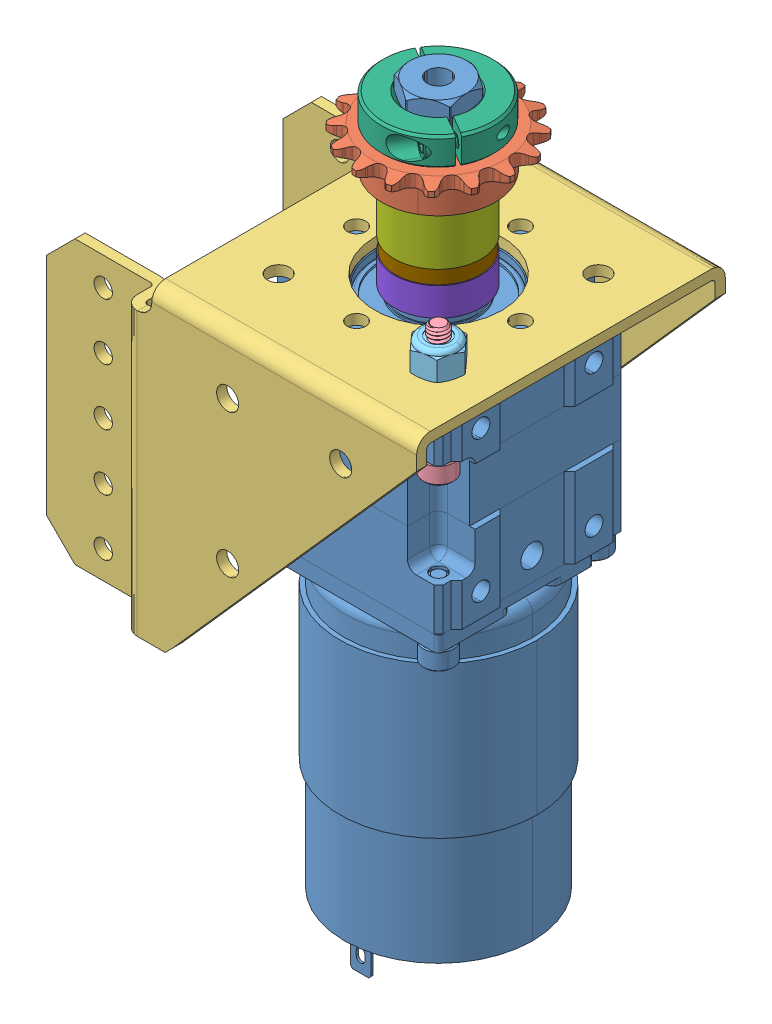
SolidWorks assembly MotorAssmb^IntakeBar, configuration Default. Lengths in mm.
Overall size (90.06 166.6 69.34).
11 component instances, 9 part files, 29 mates.
Components (placement in the parent):
- VersaPlanetary v2 Single Stage 10_1 with 775 Series -1: VersaPlanetary v2 Single Stage 10_1 with 775 Series  [Default] at (-51.9621 -18.911 -34.6718) x (0 1 0) z (0 0 -1) size (166.6 44.45 44.3)
- 16T Aluminum Hub Sprocket (#25 Chain, 1_2_ Hex Bore) (217-2642)-1: 16T Aluminum Hub Sprocket (#25 Chain, 1_2_ Hex Bore) (217-2642) [Default] at (-29.737 26.6052 -34.6572) x (0.5 0 0.866025) z (0 1 0) size (35.22 35.22 9.18)
- VersaFrame 2_ Wide VersaPlanetary Parallel Mount (217-4179)-1: VersaFrame 2_ Wide VersaPlanetary Parallel Mount (217-4179) [Default] at (-29.737 -2.286 -34.6718) x (1 0 0) z (0 1 0) size (90.06 69.34 69.72)
- 91251A199_BLACK-OXIDE ALLOY STEEL SOCKET HEAD CAP SCREW.step-1: 91251A199_BLACK-OXIDE ALLOY STEEL SOCKET HEAD CAP SCREW.step [Default] at (-11.7765 8.489 -16.7113) x (0.98845 0 -0.151546) z (0 1 0) size (6.86 6.86 29.57)
- 90631A009_LOW-STRENGTH STEEL NYLON-INSERT LOCKNUT-1: 90631A009_LOW-STRENGTH STEEL NYLON-INSERT LOCKNUT [Default] at (-11.7765 0 -16.7113) x (0.205995 0 0.978553) z (-0.978553 0 0.205995) size (8.75 5.96 10.1)
- 91251A199_BLACK-OXIDE ALLOY STEEL SOCKET HEAD CAP SCREW.step-2: 91251A199_BLACK-OXIDE ALLOY STEEL SOCKET HEAD CAP SCREW.step [Default] at (-47.6976 8.489 -52.6324) x (-0.907026 0 0.421075) z (0 1 0) size (6.86 6.86 29.57)
- 90631A009_LOW-STRENGTH STEEL NYLON-INSERT LOCKNUT-2: 90631A009_LOW-STRENGTH STEEL NYLON-INSERT LOCKNUT [Default] at (-47.6976 0 -52.6324) x (0.205995 0 0.978553) z (-0.978553 0 0.205995) size (8.75 5.96 10.1)
- WCP-0071 Rev1-1: WCP-0071 Rev1 [Default] at (-29.737 32.5742 -34.5252) x (0.866025 0 0.5) z (0 1 0) size (25.38 25.4 6.35)
- 1_2_ Acetal Spacer - 1_2_ Hex (217-3261)-1: 1_2_ Acetal Spacer - 1_2_ Hex (217-3261) [Default] at (-29.737 14.1642 -34.5252) x (0.866025 0 0.5) z (0 1 0) size (19.5 19.5 12.7)
- 1_4_ Acetal Spacer - 1_2_ Hex (217-3259)-1: 1_4_ Acetal Spacer - 1_2_ Hex (217-3259) [Default] at (-29.737 1.4642 -34.5252) x (0.866025 0 0.5) z (0 1 0) size (19.5 19.5 6.35)
- 1_8_ Acetal Spacer - 1_2_ Hex (217-2758)-1: 1_8_ Acetal Spacer - 1_2_ Hex (217-2758) [Default] at (-29.737 6.2267 -34.5252) x (1 0 0) z (0 1 0) size (19.05 19.05 3.17)
Mates (geometry in assembly coordinates):
- Coincident47: coincident anti-aligned: plane of VersaPlanetary v2 Single Stage 10_1 with 775 Series -1 through (-23.387 38.2892 -38.338) normal (0.5 0 -0.866025); plane of 16T Aluminum Hub Sprocket (#25 Chain, 1_2_ Hex Bore) (217-2642)-1 through (-23.3743 20.2224 -38.3307) normal (-0.5 0 0.866025)
- Coincident48: coincident anti-aligned: plane of VersaPlanetary v2 Single Stage 10_1 with 775 Series -1 through (-29.737 38.2892 -42.0042) normal (-0.5 0 -0.866025); plane of 16T Aluminum Hub Sprocket (#25 Chain, 1_2_ Hex Bore) (217-2642)-1 through (-29.737 20.2224 -42.0042) normal (0.5 0 0.866025)
- Distance2: distance = 8.89 mm aligned: plane of 16T Aluminum Hub Sprocket (#25 Chain, 1_2_ Hex Bore) (217-2642)-1 through (-29.737 29.3992 -34.6572) normal (0 1 0); plane of VersaPlanetary v2 Single Stage 10_1 with 775 Series -1 through (-23.387 38.2892 -38.338) normal (0 1 0)
- Coincident143: coincident anti-aligned: plane of VersaPlanetary v2 Single Stage 10_1 with 775 Series -1 through (-7.5121 -2.286 -56.8968) normal (0 1 0); plane of VersaFrame 2_ Wide VersaPlanetary Parallel Mount (217-4179)-1 through (-59.4741 -2.286 -2.286) normal (0 -1 0)
- Concentric18: concentric aligned: cylinder of VersaPlanetary v2 Single Stage 10_1 with 775 Series -1 through (-29.737 -2.286 -34.6718) axis (0 -1 0) radius 13.995; cylinder of VersaFrame 2_ Wide VersaPlanetary Parallel Mount (217-4179)-1 through (-29.737 0 -34.6718) axis (0 -1 0) radius 14.2875
- Parallel9: parallel aligned: plane of VersaPlanetary v2 Single Stage 10_1 with 775 Series -1 through (-8.737 -20.411 -25.9718) normal (1 0 0); plane of VersaFrame 2_ Wide VersaPlanetary Parallel Mount (217-4179)-1 through (0 0 -67.0577) normal (1 0 0)
- Coincident204: coincident anti-aligned: plane of VersaPlanetary v2 Single Stage 10_1 with 775 Series -1 through (-13.737 -16.911 -18.6718) normal (0 -1 0); plane of 91251A199_BLACK-OXIDE ALLOY STEEL SOCKET HEAD CAP SCREW.step-1 through (-11.7765 -16.911 -16.7113) normal (0 1 0)
- Concentric60: concentric anti-aligned: cylinder of VersaPlanetary v2 Single Stage 10_1 with 775 Series -1 through (-11.7765 -18.911 -16.7113) axis (0 -1 0) radius 2.0193; cylinder of 91251A199_BLACK-OXIDE ALLOY STEEL SOCKET HEAD CAP SCREW.step-1 through (-11.7765 -21.0766 -16.7113) axis (0 1 0) radius 3.429
- Concentric61: concentric anti-aligned: cylinder of VersaPlanetary v2 Single Stage 10_1 with 775 Series -1 through (-47.6976 -18.911 -52.6324) axis (0 -1 0) radius 2.0193; cylinder of 91251A199_BLACK-OXIDE ALLOY STEEL SOCKET HEAD CAP SCREW.step-2 through (-47.6976 -21.0766 -52.6324) axis (0 1 0) radius 3.429
- Coincident208: coincident anti-aligned: plane of VersaPlanetary v2 Single Stage 10_1 with 775 Series -1 through (-45.7371 -16.911 -50.6718) normal (0 -1 0); plane of 91251A199_BLACK-OXIDE ALLOY STEEL SOCKET HEAD CAP SCREW.step-2 through (-47.6976 -16.911 -52.6324) normal (0 1 0)
- Coincident205: coincident anti-aligned: plane of VersaFrame 2_ Wide VersaPlanetary Parallel Mount (217-4179)-1 through (-59.4741 0 -2.286) normal (0 1 0); plane of 90631A009_LOW-STRENGTH STEEL NYLON-INSERT LOCKNUT-1 through (-5.2765 0 -22.541) normal (0 -1 0)
- Coincident209: coincident anti-aligned: plane of VersaFrame 2_ Wide VersaPlanetary Parallel Mount (217-4179)-1 through (-59.4741 0 -2.286) normal (0 1 0); plane of 90631A009_LOW-STRENGTH STEEL NYLON-INSERT LOCKNUT-2 through (-41.1975 0 -58.462) normal (0 -1 0)
- Concentric58: concentric anti-aligned: cylinder of 91251A199_BLACK-OXIDE ALLOY STEEL SOCKET HEAD CAP SCREW.step-1 through (-11.7765 -16.911 -16.7113) axis (0 1 0) radius 2.0828; cylinder of 90631A009_LOW-STRENGTH STEEL NYLON-INSERT LOCKNUT-1 through (-11.7765 5.0371 -16.7113) axis (0 -1 0) radius 1.7258
- Concentric62: concentric anti-aligned: cylinder of 91251A199_BLACK-OXIDE ALLOY STEEL SOCKET HEAD CAP SCREW.step-2 through (-47.6976 -16.911 -52.6324) axis (0 1 0) radius 2.0828; cylinder of 90631A009_LOW-STRENGTH STEEL NYLON-INSERT LOCKNUT-2 through (-47.6976 5.0371 -52.6324) axis (0 -1 0) radius 1.7258
- Coincident210: coincident anti-aligned: plane of VersaPlanetary v2 Single Stage 10_1 with 775 Series -1 through (-23.387 38.2892 -38.338) normal (0.5 0 -0.866025); plane of WCP-0071 Rev1-1 through (-23.26 29.3992 -38.2647) normal (-0.5 0 0.866025)
- Coincident212: coincident anti-aligned: plane of 16T Aluminum Hub Sprocket (#25 Chain, 1_2_ Hex Bore) (217-2642)-1 through (-29.737 29.3992 -34.6572) normal (0 1 0); plane of WCP-0071 Rev1-1 through (-29.737 29.3992 -34.5252) normal (0 -1 0)
- Coincident216: coincident anti-aligned: plane of VersaPlanetary v2 Single Stage 10_1 with 775 Series -1 through (-29.737 38.2892 -42.0042) normal (-0.5 0 -0.866025); plane of WCP-0071 Rev1-1 through (-29.737 29.3992 -42.0042) normal (0.5 0 0.866025)
- Coincident242: coincident aligned: plane of VersaFrame 2_ Wide VersaPlanetary Parallel Mount (217-4179)-1 through (0 0 -67.0577) normal (1 0 0)
- Coincident243: coincident aligned: plane of VersaFrame 2_ Wide VersaPlanetary Parallel Mount (217-4179)-1 through (-62.6745 -3.1496 0) normal (0 0 1)
- Coincident244: coincident aligned: plane of VersaFrame 2_ Wide VersaPlanetary Parallel Mount (217-4179)-1 through (-59.4741 0 -2.286) normal (0 1 0)
- Coincident245: coincident anti-aligned: plane of VersaPlanetary v2 Single Stage 10_1 with 775 Series -1 through (-29.737 38.2892 -42.0042) normal (-0.5 0 -0.866025); plane of 1_2_ Acetal Spacer - 1_2_ Hex (217-3261)-1 through (-29.737 20.5142 -42.0042) normal (0.5 0 0.866025)
- Coincident246: coincident anti-aligned: plane of VersaPlanetary v2 Single Stage 10_1 with 775 Series -1 through (-23.387 38.2892 -38.338) normal (0.5 0 -0.866025); plane of 1_2_ Acetal Spacer - 1_2_ Hex (217-3261)-1 through (-23.26 20.5142 -38.2647) normal (-0.5 0 0.866025)
- Coincident203: coincident anti-aligned: plane of VersaPlanetary v2 Single Stage 10_1 with 775 Series -1 through (-29.737 38.2892 -42.0042) normal (-0.5 0 -0.866025); plane of 1_4_ Acetal Spacer - 1_2_ Hex (217-3259)-1 through (-29.737 4.6392 -42.0042) normal (0.5 0 0.866025)
- Coincident247: coincident anti-aligned: plane of VersaPlanetary v2 Single Stage 10_1 with 775 Series -1 through (-23.387 38.2892 -38.338) normal (0.5 0 -0.866025); plane of 1_4_ Acetal Spacer - 1_2_ Hex (217-3259)-1 through (-23.26 4.6392 -38.2647) normal (-0.5 0 0.866025)
- Coincident248: coincident anti-aligned: plane of VersaPlanetary v2 Single Stage 10_1 with 775 Series -1 through (-29.737 -1.7108 -34.6718) normal (0 1 0); plane of 1_4_ Acetal Spacer - 1_2_ Hex (217-3259)-1 through (-29.737 -1.7108 -34.5252) normal (0 -1 0)
- Coincident206: coincident anti-aligned: plane of VersaPlanetary v2 Single Stage 10_1 with 775 Series -1 through (-29.737 38.2892 -42.0042) normal (-0.5 0 -0.866025); plane of 1_8_ Acetal Spacer - 1_2_ Hex (217-2758)-1 through (-29.737 7.8142 -42.0042) normal (0.5 0 0.866025)
- Coincident207: coincident anti-aligned: plane of VersaPlanetary v2 Single Stage 10_1 with 775 Series -1 through (-23.387 38.2892 -38.338) normal (0.5 0 -0.866025); plane of 1_8_ Acetal Spacer - 1_2_ Hex (217-2758)-1 through (-23.26 7.8142 -38.2647) normal (-0.5 0 0.866025)
- Coincident250: coincident anti-aligned: plane of 1_2_ Acetal Spacer - 1_2_ Hex (217-3261)-1 through (-29.737 7.8142 -34.5252) normal (0 -1 0); plane of 1_8_ Acetal Spacer - 1_2_ Hex (217-2758)-1 through (-29.737 7.8142 -34.5252) normal (0 1 0)
- Coincident251: coincident anti-aligned: plane of 1_4_ Acetal Spacer - 1_2_ Hex (217-3259)-1 through (-29.737 4.6392 -34.5252) normal (0 1 0); plane of 1_8_ Acetal Spacer - 1_2_ Hex (217-2758)-1 through (-29.737 4.6392 -34.5252) normal (0 -1 0)
